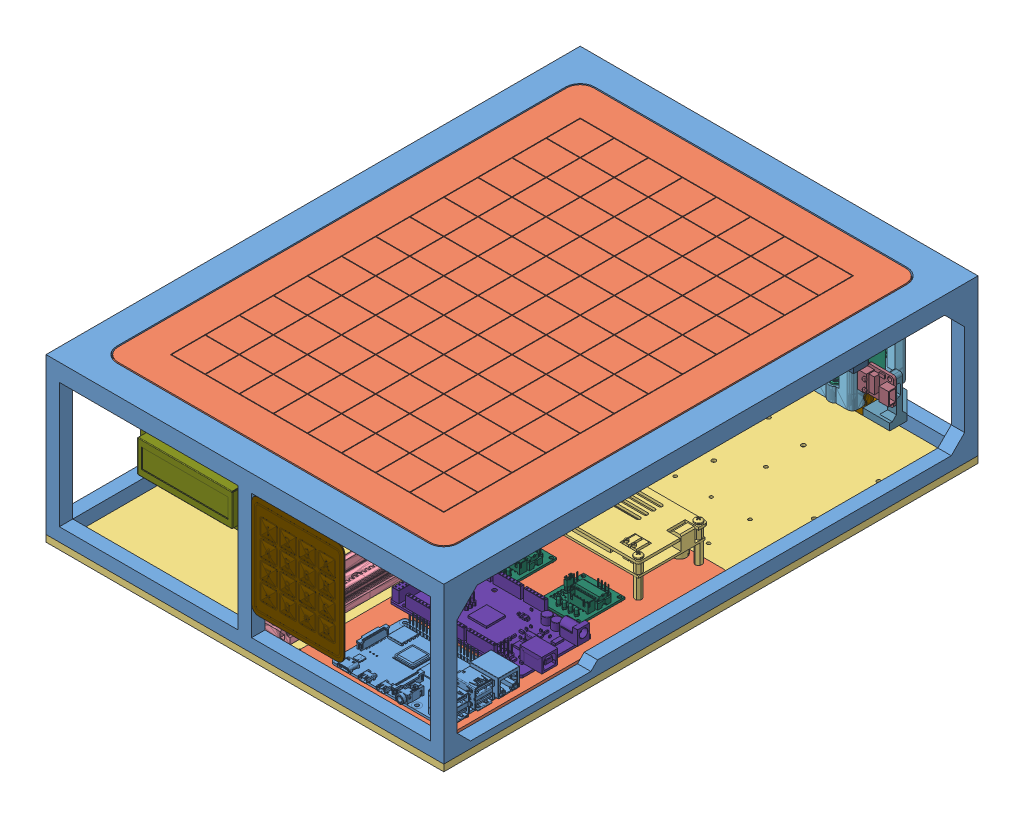
SolidWorks assembly Assembly, configuration Default. Lengths in mm.
Overall size (297.5 121.5 400.17).
29 component instances, 24 part files, 89 mates.
Components (placement in the parent):
- Frame-1: Frame [Default] at (-140.293 -41.0398 577.25) size (297.5 116.5 399.5)
- Board-1: Board [Default] at (-140.293 72.4602 577.25) size (253.5 3 355.5)
- Base-1: Base [Default] at (-162.293 -46.0398 599.25) size (297.5 5 399.5)
- GearTrackLongAxisSinglePiece-1: GearTrackLongAxisSinglePiece [Default] at (21.1485 -172.5966 584.2656) x (1 0 0) z (0 1 0) size (28 365.38 12.5)
- MotorCartMount-1: MotorCartMount [Default] at (43.5708 -25.5398 341.1932) x (-1 0 0) z (0 -1 0) size (44.96 33 30.65)
- 28BYJ-48 5V Stepper Motor-1: 28BYJ-48 5V Stepper Motor [Default] at (-13.4042 -6.5398 243.8741) x (-1 0 0) z (0 -1 0) size (42 52.5 29)
- MotorGear-1: MotorGear [Default] at (-183.9531 -37.9335 317.6846) x (0 0 -1) z (0 -1 0) size (13.6 13.6 6.5)
- AxisCartMount-1: AxisCartMount [Default] at (-34.3985 -5.5398 259.75) size (154 5 33)
- GearTrackShortAxisSinglePiece-1: GearTrackShortAxisSinglePiece [Default] at (-144.2796 -125.0068 272.4181) x (0 0 1) z (0 1 0) size (28 245.31 12.5)
- MotorCartMount-2: MotorCartMount [Default] at (187.1067 14.9602 186.2787) x (0 0 1) z (0 -1 0) size (44.96 33 30.65)
- MotorGear-2: MotorGear [Default] at (31.977 2.5665 72.7047) x (1 0 0) z (0 -1 0) size (13.6 13.6 6.5)
- 28BYJ-48 5V Stepper Motor-2: 28BYJ-48 5V Stepper Motor [Default] at (89.7876 33.9602 243.2537) x (0 0 1) z (0 -1 0) size (42 52.5 29)
- EndEffectorMountV2-1: EndEffectorMountV2 [Default] at (72.6635 32.9602 264.248) size (39 25 47)
- HK15178B-1: HK15178B [Default] at (95.0585 53.9602 274.248) x (1 0 0) z (0 1 0) size (37.75 30.2 12)
- MagnetArm-1: MagnetArm [Default] at (89.1635 53.9602 243.048) x (0 1 0) z (1 0 0) size (17.71 7 9.4)
- limit switch-1: limit switch [Default] at (116.6635 22.4602 252.248) size (26 20 11)
- ShortAxisLimitMount-1: ShortAxisLimitMount [Default] at (126.6635 4.4602 257.248) x (0 0 -1) z (0 1 0) size (28 20 33)
- limit switch-2: limit switch [Default] at (-3.543 -16.0398 215.75) x (0 0 -1) z (1 0 0) size (26 20 11)
- ULN2003-1: ULN2003 [Default] at (19.207 -36.0398 464.8338) x (1 0 0) z (0 1 0) size (31 35 11.29)
- ULN2003-2: ULN2003 [Default] at (70.207 -36.0398 464.8338) x (1 0 0) z (0 1 0) size (31 35 11.29)
- LCD_1602-1: LCD_1602 [Default] at (-54.9921 124.4602 592.5706) x (1 0 0) z (0 -1 0) size (80 17 36)
- ArduinoMega-1: ArduinoMega [Default] at (65.057 -32.3888 495.5419) x (1 0 0) z (0 -1 0) size (107.95 53.42 12.95)
- keypad-16KeyMembrane-1: keypad-16KeyMembrane [Default] at (25.9375 24.0173 599.25) x (1 0 0) z (0 -1 0) size (68.96 10.64 77.9)
- Raspberry Pi 4 Model B(CHIP SHORT REPLACEMENT)-1: Raspberry Pi 4 Model B(CHIP SHORT REPLACEMENT) [Default] at (76.707 -33.2398 555.25) size (89 19.92 58.4)
- CircuitBoardBasicDesign-1: CircuitBoardBasicDesign [Default] at (-164.793 41.9537 499.5) size (300 1.5 200) (hidden)
- ElectronicsMountingBoard-1: ElectronicsMountingBoard [Default] at (11.207 -41.0398 372.25) x (0 0 1) z (-1 0 0) size (214 4 111)
- ZK-JVA-12KX-2: ZK-JVA-12KX [Default] at (42.3358 -84.7318 444.2977) x (1 0 0) z (0 1 0) size (82 52 29.13)
- MagneticRod-1: MagneticRod [Default] at (223.8891 82.5458 284.7541) size (5.8 23.9 5.8) (hidden)
- HallEffectMount-1: HallEffectMount [Default] at (83.4275 59.4409 273.748) size (32.55 24.28 20)
Mates (geometry in assembly coordinates):
- Coincident1: coincident anti-aligned: plane of Frame-1 through (-140.293 72.4602 577.25) normal (0 1 0); plane of Board-1 through (-140.293 72.4602 577.25) normal (0 -1 0)
- Distance2: distance = 9 mm anti-aligned: plane of Board-1 through (-140.293 75.4602 221.75) normal (0 0 -1); plane of Frame-1 through (104.207 72.4602 230.75) normal (0 0 1)
- Distance3: distance = 9 mm anti-aligned: plane of Board-1 through (113.207 75.4602 577.25) normal (1 0 0); plane of Frame-1 through (104.207 72.4602 230.75) normal (-1 0 0)
- Coincident5: coincident aligned: plane of Frame-1 through (135.207 -31.0398 577.25) normal (1 0 0); plane of Base-1 through (135.207 -41.0398 599.25) normal (1 0 0)
- Coincident6: coincident anti-aligned: plane of Frame-1 through (-140.293 -41.0398 577.25) normal (0 -1 0); plane of Base-1 through (-162.293 -41.0398 599.25) normal (0 1 0)
- Coincident7: coincident aligned: plane of Frame-1 through (-140.293 -31.0398 599.25) normal (0 0 1); plane of Base-1 through (-162.293 -41.0398 599.25) normal (0 0 1)
- Coincident24: coincident: plane of Base-1 through (-162.293 -41.0398 599.25) normal (0 1 0); plane of GearTrackLongAxisSinglePiece-1 through (21.1495 -41.0398 219.6) normal (0 -1 0)
- Distance6: distance = 138.75 mm: plane of GearTrackLongAxisSinglePiece-1 through (-13.543 -172.5966 584.2656) normal (1 0 0); plane of Frame-1 through (-152.293 -31.0398 577.25) normal (1 0 0)
- Distance7: distance = 9.65 mm: plane of GearTrackLongAxisSinglePiece-1 through (-113.5428 -41.0398 579.6) normal (0 0 1); plane of Frame-1 through (-140.293 -31.0398 589.25) normal (0 0 -1)
- Concentric1: concentric anti-aligned: circle of MotorCartMount-1; circle of 28BYJ-48 5V Stepper Motor-1
- Concentric2: concentric anti-aligned: circle of MotorCartMount-1; circle of 28BYJ-48 5V Stepper Motor-1
- Coincident28: coincident anti-aligned: plane of MotorCartMount-1 through (43.5708 -25.5398 341.1932) normal (0 1 0); plane of 28BYJ-48 5V Stepper Motor-1 through (-13.4042 -25.5398 243.8741) normal (0 -1 0)
- Concentric3: concentric aligned: circle of 28BYJ-48 5V Stepper Motor-1; circle of MotorGear-1
- Parallel5: parallel anti-aligned: plane of 28BYJ-48 5V Stepper Motor-1 through (-11.4042 -35.5398 253.3741) normal (0 0 1); plane of MotorGear-1 through (-183.9531 -37.9335 253.624) normal (0 0 -1)
- Coincident30: coincident anti-aligned: plane of 28BYJ-48 5V Stepper Motor-1 through (-13.4042 -29.5398 251.8741) normal (0 -1 0); plane of MotorGear-1 through (-183.9531 -29.5398 317.6846) normal (0 1 0)
- Coincident31: coincident: plane of GearTrackLongAxisSinglePiece-1 through (-113.5428 -36.0398 376.8444) normal (0 1 0); plane of MotorGear-1 through (-183.9531 -36.0398 317.6846) normal (0 -1 0)
- Parallel6: parallel: plane of GearTrackLongAxisSinglePiece-1 through (-27.542 -172.5966 219.6) normal (-1 0 0); plane of MotorCartMount-1 through (7.456 -25.5398 341.9863) normal (1 0 0)
- Distance8: distance = 7 mm: plane of MotorCartMount-1 through (7.6015 -25.5398 341.1932) normal (1 0 0); plane of GearTrackLongAxisSinglePiece-1 through (0.456 -172.5966 219.6) normal (1 0 0)
- Coincident41: coincident: plane of MotorCartMount-1 through (43.5708 -5.5398 341.1932) normal (0 1 0); plane of AxisCartMount-1 through (-34.3985 -5.5398 259.75) normal (0 -1 0)
- Coincident43: coincident: plane of MotorCartMount-1 through (43.5708 -25.5398 226.75) normal (0 0 -1); plane of AxisCartMount-1 through (-34.3985 -0.5398 226.75) normal (0 0 -1)
- Coincident44: coincident: plane of AxisCartMount-1 through (-34.3985 -0.5398 259.75) normal (0 1 0); plane of GearTrackShortAxisSinglePiece-1 through (106.5315 -0.5398 257.248) normal (0 -1 0)
- Distance9: distance = 2.5 mm: plane of GearTrackShortAxisSinglePiece-1 through (106.5315 4.2102 229.25) normal (0 0 -1); plane of AxisCartMount-1 through (-34.3985 -0.5398 226.75) normal (0 0 -1)
- Distance12: distance = 99.07 mm: plane of MotorCartMount-1 through (-34.3985 -25.5398 341.1932) normal (-1 0 0); plane of GearTrackShortAxisSinglePiece-1 through (-133.4685 -125.0068 272.4181) normal (-1 0 0)
- Distance13: distance = 60 mm: plane of MotorCartMount-1 through (-34.3985 -25.5398 341.1932) normal (-1 0 0); plane of AxisCartMount-1 through (-94.3985 -5.5398 259.75) normal (-1 0 0)
- Concentric4: concentric anti-aligned: circle of MotorCartMount-2; circle of 28BYJ-48 5V Stepper Motor-2
- Concentric5: concentric anti-aligned: circle of MotorCartMount-2; circle of 28BYJ-48 5V Stepper Motor-2
- Coincident45: coincident anti-aligned: plane of MotorCartMount-2 through (187.1067 14.9602 186.2787) normal (0 1 0); plane of 28BYJ-48 5V Stepper Motor-2 through (89.7876 14.9602 243.2537) normal (0 -1 0)
- Concentric6: concentric aligned: circle of MotorGear-2; circle of 28BYJ-48 5V Stepper Motor-2
- Parallel7: parallel anti-aligned: plane of MotorGear-2 through (96.0376 2.5665 72.7047) normal (1 0 0); plane of 28BYJ-48 5V Stepper Motor-2 through (96.2876 4.9602 245.2537) normal (-1 0 0)
- Coincident47: coincident anti-aligned: plane of MotorGear-2 through (31.977 10.9602 72.7047) normal (0 1 0); plane of 28BYJ-48 5V Stepper Motor-2 through (97.7876 10.9602 243.2537) normal (0 -1 0)
- Coincident48: coincident: plane of GearTrackShortAxisSinglePiece-1 through (-170.8449 4.4602 143.2503) normal (0 1 0); plane of MotorGear-2 through (31.977 4.4602 72.7047) normal (0 -1 0)
- Distance14: distance = 7 mm: plane of MotorCartMount-2 through (187.1067 14.9602 264.248) normal (0 0 1); plane of GearTrackShortAxisSinglePiece-1 through (106.5315 4.2102 257.248) normal (0 0 1)
- Coincident50: coincident aligned: plane of MotorCartMount-2 through (105.6635 14.9602 186.2787) normal (1 0 0); plane of EndEffectorMountV2-1 through (105.6635 37.9602 264.248) normal (1 0 0)
- Coincident51: coincident: plane of MotorCartMount-2 through (187.1067 34.9602 186.2787) normal (0 1 0); plane of EndEffectorMountV2-1 through (-96.9432 34.9602 103.4217) normal (0 -1 0)
- Coincident58: coincident anti-aligned: plane of HK15178B-1 through (89.1635 53.9602 250.048) normal (0 0 -1); plane of MagnetArm-1 through (89.1635 53.9602 250.048) normal (0 0 1)
- Concentric8: concentric: circle of HK15178B-1; circle of MagnetArm-1
- Coincident66: coincident aligned: plane of MotorCartMount-2 through (187.1067 14.9602 222.248) normal (0 0 -1); plane of EndEffectorMountV2-1 through (72.6635 37.9602 222.248) normal (0 0 -1)
- Coincident67: coincident: plane of EndEffectorMountV2-1 through (72.6635 47.9602 264.248) normal (0 1 0); plane of HK15178B-1 through (83.5585 47.9602 263.748) normal (0 -1 0)
- Parallel14: parallel: plane of EndEffectorMountV2-1 through (72.6635 47.9602 264.248) normal (0 1 0); plane of MagnetArm-1 through (89.1635 66.9702 243.048) normal (0 1 0)
- Distance21: distance = 16.5 mm: line of HK15178B-1 through (89.1635 47.9602 250.048) axis (0 0 1); line of EndEffectorMountV2-1 through (72.6635 47.9602 256.7573) axis (0 0 1)
- Coincident69: coincident: plane of EndEffectorMountV2-1 through (111.6635 57.9602 263.748) normal (0 0 -1); plane of HK15178B-1 through (95.0585 53.9602 263.748) normal (0 0 1)
- Coincident70: coincident anti-aligned: plane of GearTrackShortAxisSinglePiece-1 through (106.6635 -0.5398 143.2503) normal (1 0 0); plane of limit switch-1 through (106.6635 32.4602 254.248) normal (-1 0 0)
- Distance22: distance = 3 mm aligned: plane of limit switch-1 through (116.6635 22.4602 260.248) normal (0 0 1); plane of GearTrackShortAxisSinglePiece-1 through (106.5315 4.2102 257.248) normal (0 0 1)
- Distance23: distance = 13 mm anti-aligned: plane of limit switch-1 through (105.6635 17.4602 260.248) normal (0 -1 0); plane of GearTrackShortAxisSinglePiece-1 through (-50.7789 4.4602 143.2503) normal (0 1 0)
- Coincident78: coincident aligned: plane of GearTrackShortAxisSinglePiece-1 through (106.5315 4.2102 257.248) normal (0 0 1); plane of ShortAxisLimitMount-1 through (106.6635 4.4602 257.248) normal (0 0 1)
- Coincident79: coincident aligned: plane of GearTrackShortAxisSinglePiece-1 through (-50.7789 4.4602 143.2503) normal (0 1 0); plane of ShortAxisLimitMount-1 through (106.6635 4.4602 257.248) normal (0 1 0)
- Coincident80: coincident anti-aligned: line of GearTrackShortAxisSinglePiece-1 through (106.6635 4.4602 237.02) axis (0 0 1); line of ShortAxisLimitMount-1 through (106.6635 4.4602 257.248) axis (0 0 -1)
- Distance27: distance = 17 mm: plane of limit switch-2 through (4.457 -8.0398 226.75) normal (0 0 1); plane of Frame-1 through (-140.293 -31.0398 209.75) normal (0 0 1)
- Distance28: distance = 5 mm: plane of limit switch-2 through (-3.543 -16.0398 215.75) normal (-1 0 0); plane of Frame-1 through (-8.543 62.4602 209.75) normal (1 0 0)
- Distance29: distance = 15 mm: plane of Base-1 through (-162.293 -41.0398 599.25) normal (0 1 0); plane of limit switch-2 through (-1.543 -26.0398 225.75) normal (0 -1 0)
- Distance32: distance = 5 mm: plane of ULN2003-1 through (19.207 -36.0398 464.8338) normal (0 -1 0); plane of Base-1 through (-162.293 -41.0398 599.25) normal (0 1 0)
- Distance33: distance = 5 mm: plane of ULN2003-2 through (70.207 -36.0398 464.8338) normal (0 -1 0); plane of Base-1 through (-162.293 -41.0398 599.25) normal (0 1 0)
- Coincident81: coincident: plane of Base-1 through (-162.293 -41.0398 599.25) normal (0 1 0); plane of ElectronicsMountingBoard-1 through (11.207 -41.0398 372.25) normal (0 -1 0)
- Parallel16: parallel anti-aligned: plane of Frame-1 through (135.207 -31.0398 577.25) normal (1 0 0); plane of ElectronicsMountingBoard-1 through (11.207 -37.0398 372.25) normal (-1 0 0)
- Distance34: distance = 3 mm: plane of Raspberry Pi 4 Model B(CHIP SHORT REPLACEMENT)-1 through (76.707 -34.0398 555.25) normal (0 -1 0); plane of ElectronicsMountingBoard-1 through (11.207 -37.0398 372.25) normal (0 1 0)
- Coincident84: coincident: plane of Raspberry Pi 4 Model B(CHIP SHORT REPLACEMENT)-1 through (122.207 -25.6898 537.5) normal (1 0 0); plane of ElectronicsMountingBoard-1 through (122.207 -37.0398 372.25) normal (1 0 0)
- Distance36: distance = 3 mm: plane of ArduinoMega-1 through (115.857 -34.0398 468.8338) normal (0 -1 0); plane of ElectronicsMountingBoard-1 through (11.207 -37.0398 372.25) normal (0 1 0)
- Coincident87: coincident: plane of ArduinoMega-1 through (122.207 -21.5938 512.979) normal (1 0 0); plane of ElectronicsMountingBoard-1 through (122.207 -37.0398 372.25) normal (1 0 0)
- Coincident88: coincident anti-aligned: plane of ElectronicsMountingBoard-1 through (11.207 -37.0398 372.25) normal (0 1 0); plane of ZK-JVA-12KX-2 through (104.207 -37.0398 375.1519) normal (0 -1 0)
- Distance37: distance = 3 mm aligned: plane of ZK-JVA-12KX-2 through (106.707 -20.4398 375.25) normal (0 0 -1); plane of ElectronicsMountingBoard-1 through (11.207 -37.0398 372.25) normal (0 0 -1)
- Distance38: distance = 3 mm: plane of Raspberry Pi 4 Model B(CHIP SHORT REPLACEMENT)-1 through (34.207 -32.4398 583.25) normal (0 0 1); plane of ElectronicsMountingBoard-1 through (11.207 -37.0398 586.25) normal (0 0 1)
- Distance39: distance = 15.5 mm: plane of ZK-JVA-12KX-2 through (106.707 -20.4398 425.25) normal (1 0 0); plane of ElectronicsMountingBoard-1 through (122.207 -37.0398 372.25) normal (1 0 0)
- Distance40: distance = 5 mm: plane of ArduinoMega-1 through (14.257 -34.0398 522.25) normal (0 0 1); plane of Raspberry Pi 4 Model B(CHIP SHORT REPLACEMENT)-1 through (34.207 -32.4398 527.25) normal (0 0 -1)
- Coincident96: coincident aligned: plane of ULN2003-1 through (19.207 -36.0398 464.8338) normal (0 0 1); plane of ULN2003-2 through (70.207 -36.0398 464.8338) normal (0 0 1)
- Distance41: distance = 20 mm: plane of ULN2003-1 through (50.207 -36.0398 464.8338) normal (1 0 0); plane of ULN2003-2 through (70.207 -36.0398 429.8338) normal (-1 0 0)
- Distance42: distance = 4 mm anti-aligned: plane of ULN2003-2 through (70.207 -36.0398 464.8338) normal (0 0 1); plane of ArduinoMega-1 through (14.257 -34.0398 468.8338) normal (0 0 -1)
- Distance43: distance = 8 mm: plane of ElectronicsMountingBoard-1 through (11.207 -37.0398 372.25) normal (-1 0 0); plane of ULN2003-1 through (19.207 -36.0398 429.8338) normal (-1 0 0)
- Distance44: distance = 3 mm: plane of ElectronicsMountingBoard-1 through (11.207 -37.0398 586.25) normal (0 0 1); plane of Frame-1 through (-140.293 -31.0398 589.25) normal (0 0 -1)
- Distance45: distance = 3 mm: plane of ElectronicsMountingBoard-1 through (122.207 -37.0398 372.25) normal (1 0 0); plane of Frame-1 through (125.207 -31.0398 577.25) normal (-1 0 0)
- Parallel20: parallel aligned: plane of Frame-1 through (135.207 -31.0398 577.25) normal (1 0 0); plane of CircuitBoardBasicDesign-1 through (135.207 43.4537 499.5) normal (1 0 0)
- Parallel21: parallel aligned: plane of Frame-1 through (-140.293 75.4602 577.25) normal (0 1 0); plane of CircuitBoardBasicDesign-1 through (-164.793 43.4537 499.5) normal (0 1 0)
- Coincident107: coincident aligned: plane of Frame-1 through (135.207 -31.0398 577.25) normal (1 0 0); plane of CircuitBoardBasicDesign-1 through (135.207 43.4537 499.5) normal (1 0 0)
- Distance47: distance = 1.75 mm aligned: plane of Board-1 through (63.207 74.9602 297.75) normal (0 0 -1); plane of CircuitBoardBasicDesign-1 through (-164.793 43.4537 299.5) normal (0 0 -1)
- Coincident110: coincident aligned: plane of Frame-1 through (-140.293 -31.0398 599.25) normal (0 0 1); plane of keypad-16KeyMembrane-1 through (25.9375 24.0173 599.25) normal (0 0 1)
- Coincident111: coincident anti-aligned: plane of Frame-1 through (-140.293 62.4602 577.25) normal (0 -1 0); plane of keypad-16KeyMembrane-1 through (55.338 62.4602 599.25) normal (0 1 0)
- Coincident112: coincident aligned: plane of Frame-1 through (-140.293 -31.0398 599.25) normal (0 0 1); plane of LCD_1602-1 through (-94.043 31.8602 599.25) normal (0 0 1)
- Parallel22: parallel anti-aligned: plane of Frame-1 through (-140.293 -31.0398 577.25) normal (0 1 0); plane of LCD_1602-1 through (-98.543 26.4602 592.25) normal (0 -1 0)
- Coincident114: coincident anti-aligned: plane of Frame-1 through (-18.543 62.4602 599.25) normal (-1 0 0); plane of LCD_1602-1 through (-18.543 26.4602 592.25) normal (1 0 0)
- Coincident115: coincident anti-aligned: plane of Frame-1 through (-140.293 62.4602 577.25) normal (0 -1 0); plane of LCD_1602-1 through (-98.543 62.4602 592.25) normal (0 1 0)
- Coincident116: coincident anti-aligned: plane of Frame-1 through (-8.543 62.4602 599.25) normal (1 0 0); plane of keypad-16KeyMembrane-1 through (-8.543 57.3802 599.25) normal (-1 0 0)
- Coincident117: coincident: plane of Base-1 through (-162.293 -41.0398 599.25) normal (0 1 0); plane of GearTrackLongAxisSinglePiece-1 through (-113.5428 -41.0398 616.9764) normal (0 -1 0)
- Distance48: distance = 124.75 mm: plane of Frame-1 through (-152.293 -31.0398 577.25) normal (1 0 0); plane of GearTrackLongAxisSinglePiece-1 through (-27.543 -41.0398 496.9104) normal (-1 0 0)
- Coincident118: coincident: plane of HK15178B-1 through (83.5585 59.9602 263.748) normal (0 1 0); plane of HallEffectMount-1 through (84.3303 58.6845 296.2654) normal (0 -1 0)
- Coincident119: coincident: plane of HK15178B-1 through (106.5585 59.9602 263.748) normal (1 0 0); plane of HallEffectMount-1 through (106.4275 62.4409 273.748) normal (1 0 0)
- Coincident120: coincident: plane of HK15178B-1 through (95.0585 53.9602 263.748) normal (0 0 1); plane of HallEffectMount-1 through (83.4275 62.4409 263.748) normal (0 0 -1)
- Coincident123: coincident: plane of MotorCartMount-1 through (43.5708 -25.5398 226.75) normal (0 0 -1); plane of limit switch-2 through (4.457 -8.0398 226.75) normal (0 0 1)
- Coincident124: coincident anti-aligned: plane of MotorCartMount-2 through (105.6635 14.9602 186.2787) normal (1 0 0); plane of limit switch-1 through (105.6635 30.4602 260.248) normal (-1 0 0)
- Coincident125: coincident anti-aligned: plane of MotorCartMount-2 through (187.1067 34.9602 186.2787) normal (0 1 0); plane of EndEffectorMountV2-1 through (109.6635 34.9602 258.7573) normal (0 -1 0)
- Concentric9: concentric: circle of EndEffectorMountV2-1; circle of HallEffectMount-1
